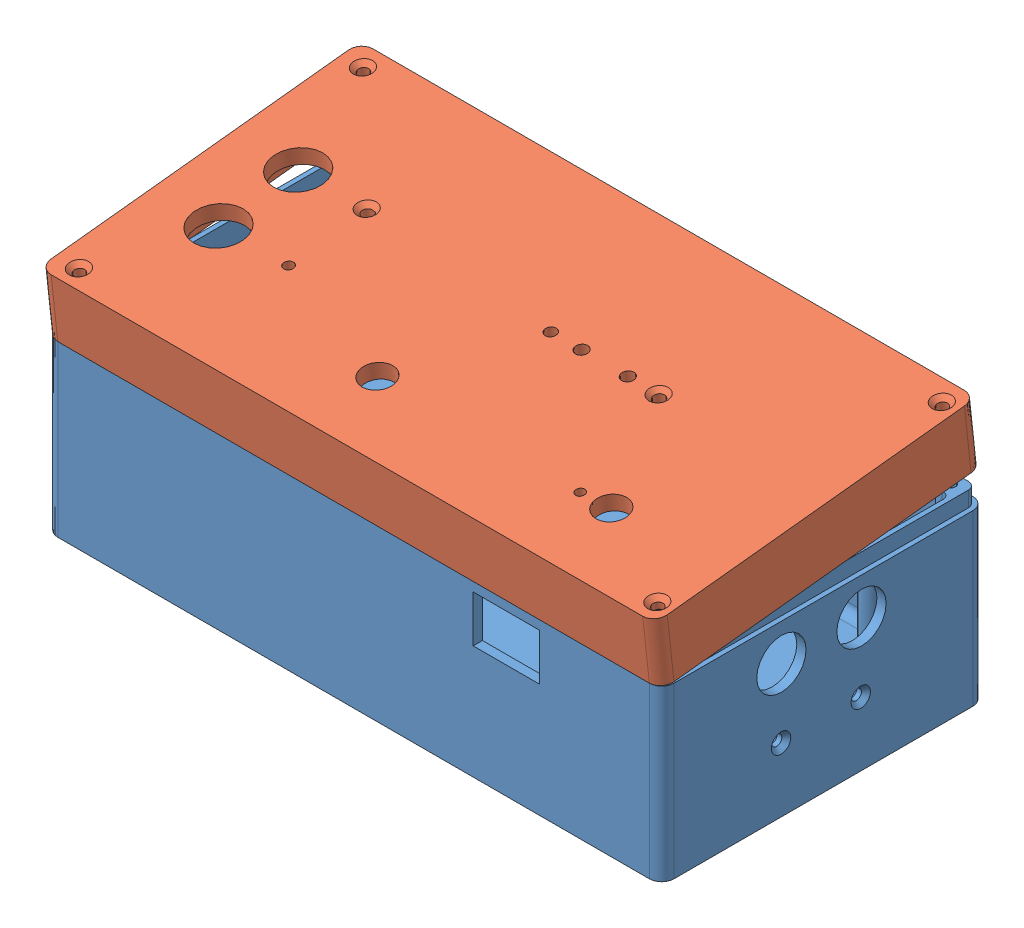
SolidWorks assembly Assemblage_Boitier+Couvercle, configuration Default. Lengths in mm.
Overall size (203 86.37 110.15).
2 component instances, 2 part files, 3 mates.
Components (placement in the parent):
- Theremin-Boitier_JonathanCHAFLA-1: Theremin-Boitier_JonathanCHAFLA [Default] at (-1328.4654 62.0969 1104.789) size (203 60 108)
- Theremin-Boitier_JonathanCHAFLA-Couvercle-1: Theremin-Boitier_JonathanCHAFLA-Couvercle [Default] at (-1327.4934 138.0275 1100.7748) x (1 0 0) z (0 0.107836 -0.994169) size (203 20 108)
Mates (geometry in assembly coordinates):
- Coïncidente76: coincident anti-aligned: line of Theremin-Boitier_JonathanCHAFLA-1 through (-1403.4637 117.0969 1154.6396) axis (1 0 0); line of Theremin-Boitier_JonathanCHAFLA-Couvercle-1 through (-1211.4637 117.0969 1154.6396) axis (-1 0 0)
- Coïncidente77: coincident aligned: plane of Theremin-Boitier_JonathanCHAFLA-1 through (-1207.4637 122.0969 1049.6396) normal (1 0 0); plane of Theremin-Boitier_JonathanCHAFLA-Couvercle-1 through (-1207.4637 136.9802 1156.7963) normal (1 0 0)
- Coïncidente80: coincident aligned: circle of Theremin-Boitier_JonathanCHAFLA-Couvercle-1; plane of Potentiometer-1 through (-1320.2674 145.4627 1160.4306) normal (0 0.336561 0.941662)
